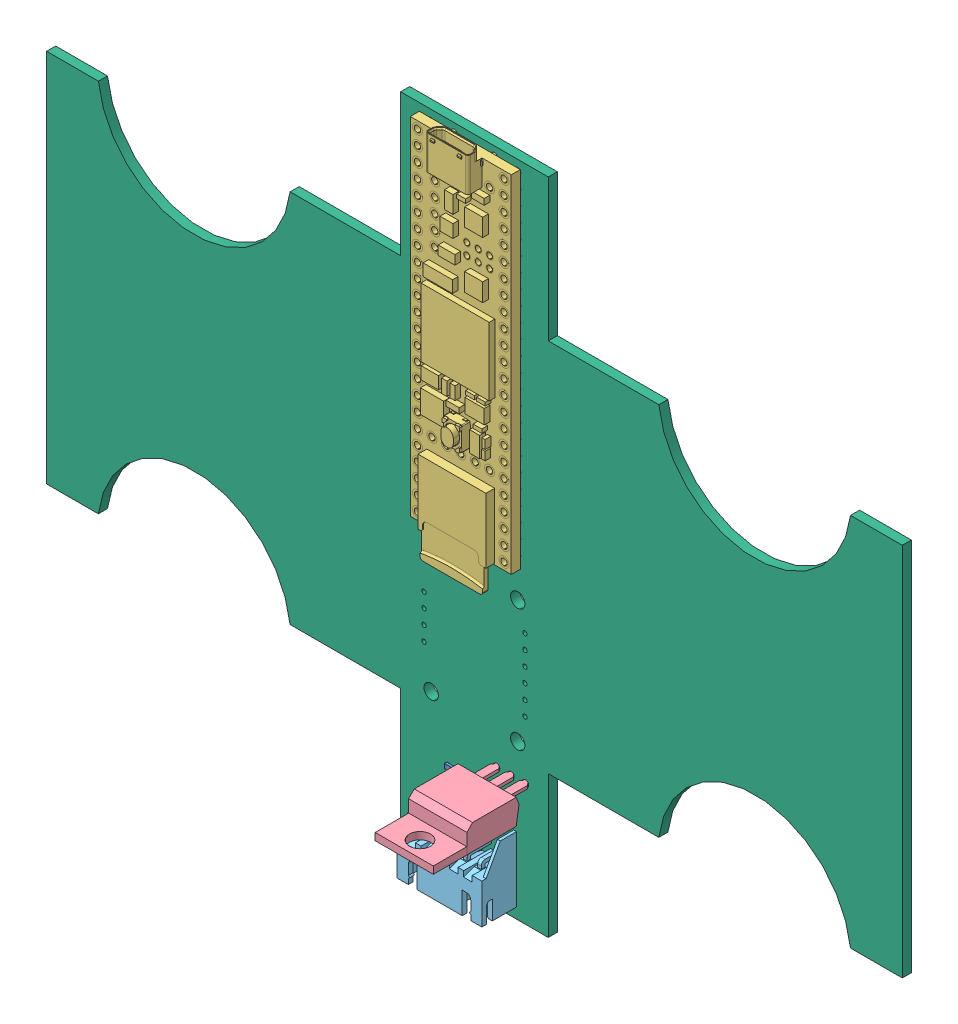
SolidWorks assembly microtaur-teensy41, configuration Default. Lengths in mm.
Overall size (150.7 116.98 28.52).
14 component instances, 6 part files, 0 mates.
Components (placement in the parent):
- microtaur-teensy41.step-1: microtaur-teensy41.step [Default] at origin size (150.7 116.98 28.52)
  - R_0603_1608Metric.step-1: R_0603_1608Metric.step [Default] at (-4 -40.5 1.65) x (-1 0 0) z (0 0 1) size (1.6 0.8 0.45)
    - SOLID.step-1: SOLID.step [Default] at origin size (1.6 0.8 0.45)
  - R_0603_1608Metric.step-2: R_0603_1608Metric.step [Default] at (-0.5 -40.5 1.65) x (-1 0 0) z (0 0 1) size (1.6 0.8 0.45)
    - SOLID.step-1: SOLID.step [Default] at origin size (1.6 0.8 0.45)
  - C_0805_2012Metric.step-1: C_0805_2012Metric.step [Default] at (-2 -43.5 1.65) x (-1 0 0) z (0 0 1) size (2 1.25 1.25)
    - SOLID-0.step-1: SOLID-0.step [Default] at origin size (2 1.25 1.25)
  - Teensy_4.1_Assembly.step-1: Teensy_4.1_Assembly.step [Default] at (0 27 2.412) x (0 -1 0) z (0 0 1) size (66.56 17.78 5.27)
    - COMPOUND.step-1: COMPOUND.step [Default] at origin size (66.56 17.78 5.27)
  - TO-220-3_Vertical.step-1: TO-220-3_Vertical.step [Default] at (9 -36.5 1.65) x (-1 0 0) z (0 0 1) size (10.25 4.46 28.53)
    - SOLID-1.step-1: SOLID-1.step [Default] at origin size (10.25 4.46 28.53)
  - JST_XH_S5B-XH-A-1_1x05_P2.50mm_Horizontal.step-1: JST_XH_S5B-XH-A-1_1x05_P2.50mm_Horizontal.step [Default] at (-5 -48.5 1.65) size (14.9 11.5 9.5)
    - SOLID-2.step-1: SOLID-2.step [Default] at origin size (14.9 11.5 9.5)
  - COMPOUND-3.step-1: COMPOUND-3.step [Default] at origin size (150.7 116 1.6)
